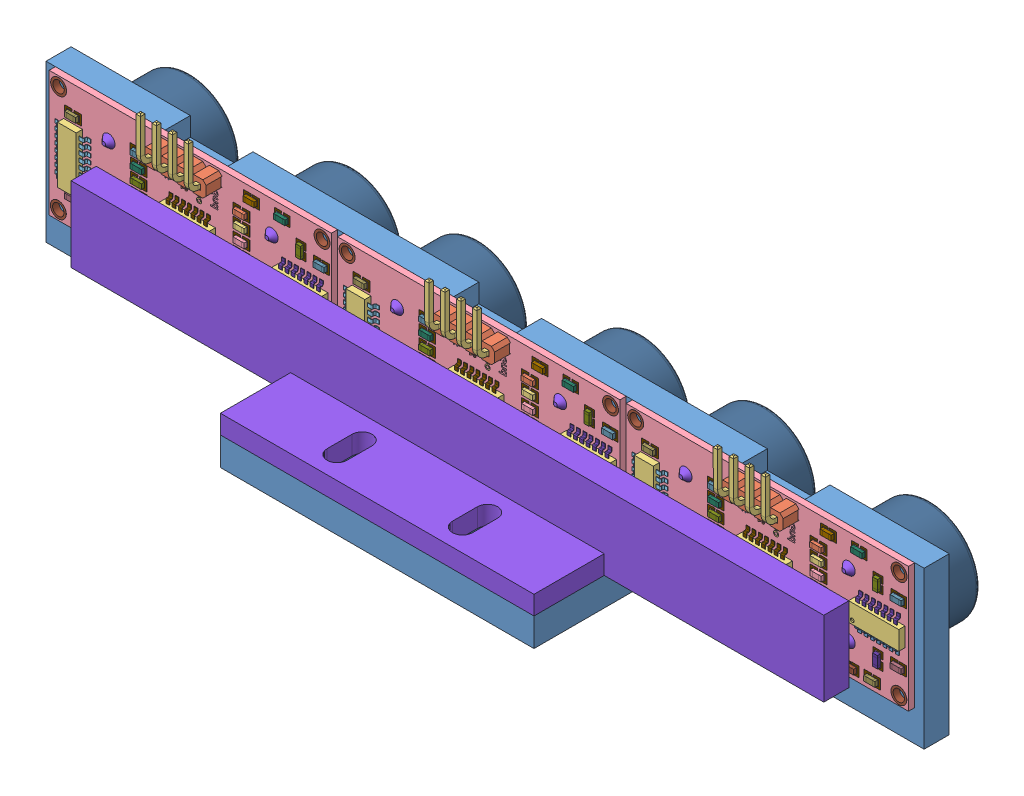
SolidWorks assembly Assem4, configuration Default. Lengths in mm.
Overall size (140 30.57 29.2).
188 component instances, 62 part files, 9 mates.
Components (placement in the parent):
- ga lap ultrasonic v5-1: ga lap ultrasonic v5 [Default] at (40.1597 76.4517 111.5417) size (140 25 21.2)
- HC-04HC-04-1: HC-04HC-04 [Default] at (54.2402 85.1585 116.5417) x (1 0 0) z (0 0 -1) size (45 25.57 17.46)
  - HC-04HC-04.stp-1: HC-04HC-04.stp [Default] at origin size (45 25.57 17.46)
    - HC-04Array.stp-1: HC-04Array.stp [Default] at origin size (10.16 2.54 2.54)
    - HC-04Array001.stp-1: HC-04Array001.stp [Default] at (0 0 1) size (8.32 7.52 6.46)
    - HC-04Placa.stp-1: HC-04Placa.stp [Default] at origin size (45 20 1)
    - HC-04Pad003.stp-1: HC-04Pad003.stp [Default] at (0 0 1) size (10.52 3.38 0.2)
    - HC-04Fillet.stp-1: HC-04Fillet.stp [Default] at (0 0 1) size (10.1 2.84 3)
    - HC-04Array002.stp-1: HC-04Array002.stp [Default] at origin size (9.62 2 1)
    - HC-04Array003.stp-1: HC-04Array003.stp [Default] at (0 0 1) size (28 12 0.8)
    - HC-04Fusion.stp-1: HC-04Fusion.stp [Default] at origin size (6 2 1)
    - HC-04Fillet001.stp-1: HC-04Fillet001.stp [Default] at (0 0 1) size (42 16 12)
    - HC-04Pad005.stp-1: HC-04Pad005.stp [Default] at (0 0 1) size (39.16 13 0.2)
    - HC-04Pad006.stp-1: HC-04Pad006.stp [Default] at (0 0 1) size (35.01 9.04 7)
    - HC-04Fusion001.stp-1: HC-04Fusion001.stp [Default] at (0 0 8) size (31 5 1.5)
    - HC-04Clone_of_Fusion002.stp-1: HC-04Clone_of_Fusion002.stp [Default] at (47.2 -5.5 12.6) size (13 13 0.15)
    - HC-04Clone_of_Fusion003.stp-1: HC-04Clone_of_Fusion003.stp [Default] at (21.2 -5.5 12.6) size (13 13 0.15)
    - HC-04Array005.stp-1: HC-04Array005.stp [Default] at origin size (9.62 2 1)
    - HC-04Array002002.stp-1: HC-04Array002002.stp [Default] at (-5.9 0.1 0.15) size (6.57 1.4 0.56)
    - HC-04Clone_of_Array002002.stp-1: HC-04Clone_of_Array002002.stp [Default] at (-23.9 0.1 0.15) size (6.57 1.4 0.56)
    - HC-04Array002003.stp-1: HC-04Array002003.stp [Default] at (-6.05 0 0.15) size (6.57 1.4 0.56)
    - HC-04Clone_of_Array002003.stp-1: HC-04Clone_of_Array002003.stp [Default] at (-24.05 0 0.15) size (6.57 1.4 0.56)
    - HC-04Integrados.stp-1: HC-04Integrados.stp [Default] at origin size (42.14 9 1)
    - HC-04ShapeString.stp-1: HC-04ShapeString.stp [Default] at (-3.2 -7 1.01) x (0 1 0) z (0 0 1) size (2.53 1.13 0.01)
    - HC-04ShapeString001.stp-1: HC-04ShapeString001.stp [Default] at (-0.6 -7 1.01) x (0 1 0) z (0 0 1) size (2.66 1.45 0.01)
    - HC-04ShapeString002.stp-1: HC-04ShapeString002.stp [Default] at (1.9 -7 1.01) x (0 1 0) z (0 0 1) size (3.21 1.16 0.01)
    - HC-04ShapeString003.stp-1: HC-04ShapeString003.stp [Default] at (4.5 -7 1.01) x (0 1 0) z (0 0 1) size (2.71 1.16 0.01)
    - HC-04ShapeString004.stp-1: HC-04ShapeString004.stp [Default] at (-19.5 -9.3 1.01) size (1.84 2.34 0.01)
    - HC-04ShapeString005.stp-1: HC-04ShapeString005.stp [Default] at (17.5 -9.3 1.01) size (1.82 2.34 0.01)
    - HC-04ShapeString006.stp-1: HC-04ShapeString006.stp [Default] at (-3 3.7 1.01) size (5.52 1.41 0.01)
    - HC-04Pad008.stp-1: HC-04Pad008.stp [Default] at (0 0 -0.01) size (44.56 19.6 1.02)
    - HC-04Scale004.stp-1: HC-04Scale004.stp [Default] at (-1.9 -21.5 -1.5) x (0 1 0) z (0 0 1) size (0.8 1.77 0.5)
    - HC-04Scale027.stp-1: HC-04Scale027.stp [Default] at (-1.9 -10.2323 -1.5) x (0 1 0) z (0 0 1) size (0.8 1.77 0.5)
    - HC-04Scale028.stp-1: HC-04Scale028.stp [Default] at (8.5984 -21.5 -1.5) x (0 1 0) z (0 0 1) size (0.8 1.77 0.5)
    - HC-04Scale029.stp-1: HC-04Scale029.stp [Default] at (8.5984 -19.5867 -1.5) x (0 1 0) z (0 0 1) size (0.8 1.77 0.5)
    - HC-04Scale030.stp-1: HC-04Scale030.stp [Default] at (8.5984 -17.5982 -1.5) x (0 1 0) z (0 0 1) size (0.8 1.77 0.5)
    - HC-04Scale031.stp-1: HC-04Scale031.stp [Default] at (8.5984 -15.6427 -1.5) x (0 1 0) z (0 0 1) size (0.8 1.77 0.5)
    - HC-04Scale032.stp-1: HC-04Scale032.stp [Default] at (8.5984 -11.6848 -1.5) x (0 1 0) z (0 0 1) size (0.8 1.77 0.5)
    - HC-04Scale033.stp-1: HC-04Scale033.stp [Default] at (-26.74 -2 -1.5) x (0 1 0) z (0 0 1) size (0.8 1.85 0.5)
    - HC-04Scale034.stp-1: HC-04Scale034.stp [Default] at (24.9371 -21.5 -1.5) x (0 1 0) z (0 0 1) size (0.8 1.77 0.5)
    - HC-04Scale035.stp-1: HC-04Scale035.stp [Default] at (24.9691 -19.5867 -1.5) x (0 1 0) z (0 0 1) size (0.8 1.77 0.5)
    - HC-04Scale036.stp-1: HC-04Scale036.stp [Default] at (24.9742 -17.5982 -1.5) x (0 1 0) z (0 0 1) size (0.8 1.77 0.5)
    - HC-04Scale037.stp-1: HC-04Scale037.stp [Default] at (-10.4013 -2 -1.5) x (0 1 0) z (0 0 1) size (0.8 1.85 0.5)
    - HC-04Scale038.stp-1: HC-04Scale038.stp [Default] at (-10.4013 -3.9266 -1.5) x (0 1 0) z (0 0 1) size (0.8 1.85 0.5)
    - HC-04Scale039.stp-1: HC-04Scale039.stp [Default] at (-10.4013 -0.0734 -1.5) x (0 1 0) z (0 0 1) size (0.8 1.85 0.5)
    - HC-04Scale040.stp-1: HC-04Scale040.stp [Default] at (24.9742 -9.855 -1.5) x (0 1 0) z (0 0 1) size (0.8 1.77 0.5)
    - HC-04Scale041.stp-1: HC-04Scale041.stp [Default] at (26.5673 -24.0564 -1.5) x (0 1 0) z (0 0 1) size (0.8 1.77 0.5)
    - HC-04Scale042.stp-1: HC-04Scale042.stp [Default] at (26.5673 -7.3333 -1.5) x (0 1 0) z (0 0 1) size (0.8 1.77 0.5)
    - HC-04Scale043.stp-1: HC-04Scale043.stp [Default] at (30.1435 -7.3333 -1.5) x (0 1 0) z (0 0 1) size (0.8 1.77 0.5)
    - HC-04Scale044.stp-1: HC-04Scale044.stp [Default] at (33.5459 -7.3333 -1.5) x (0 1 0) z (0 0 1) size (0.8 1.77 0.5)
    - HC-04Scale045.stp-1: HC-04Scale045.stp [Default] at (37.7181 -11.1827 -1.5) x (0 1 0) z (0 0 1) size (0.8 1.77 0.5)
    - HC-04Scale046.stp-1: HC-04Scale046.stp [Default] at (37.7181 -20.5932 -1.5) x (0 1 0) z (0 0 1) size (0.8 1.77 0.5)
    - HC-04Scale047.stp-1: HC-04Scale047.stp [Default] at (-3.9042 -12.3288 -1.5) x (0 1 0) z (0 0 1) size (0.8 1.85 0.5)
    - HC-04Scale048.stp-1: HC-04Scale048.stp [Default] at (13.5402 13.2894 -1.5) size (0.8 1.85 0.5)
    - HC-04Scale049.stp-1: HC-04Scale049.stp [Default] at (13.5402 23.7909 -1.5) size (0.8 1.85 0.5)
    - HC-04Pad009.stp-1: HC-04Pad009.stp [Default] x (1 0 0) z (0 0 -1) size (42.21 18.43 0.01)
    - HC-04ShapeString007.stp-1: HC-04ShapeString007.stp [Default] at (-3.2 -7 -0.1) x (0 1 0) z (0 0 1) size (2.53 1.13 0.01)
    - HC-04ShapeString008.stp-1: HC-04ShapeString008.stp [Default] at (-0.6 -7 -0.1) x (0 1 0) z (0 0 1) size (2.66 1.45 0.01)
    - HC-04ShapeString009.stp-1: HC-04ShapeString009.stp [Default] at (1.9 -7 -0.1) x (0 1 0) z (0 0 1) size (3.21 1.16 0.01)
    - HC-04ShapeString010.stp-1: HC-04ShapeString010.stp [Default] at (4.5 -7 -0.1) x (0 1 0) z (0 0 1) size (2.71 1.16 0.01)
    - HC-04Fusion002.stp-1: HC-04Fusion002.stp [Default] at origin size (5.7 7.57 0.56)
    - HC-04ShapeString011.stp-1: HC-04ShapeString011.stp [Default] at (-17.5 8.4 1.1) size (7.91 1.16 0.01)
    - HC-04ShapeString012.stp-1: HC-04ShapeString012.stp [Default] at (-7.5 8 -0.1) x (-1 0 0) z (0 0 -1) size (7.91 1.16 0.01)
- HC-04HC-04-2: HC-04HC-04 [Default] at (100.2402 85.1585 116.5417) x (1 0 0) z (0 0 -1) size (45 25.57 17.46)
  - HC-04HC-04.stp-1: HC-04HC-04.stp [Default] at origin size (45 25.57 17.46)
    - HC-04Array.stp-1: HC-04Array.stp [Default] at origin size (10.16 2.54 2.54)
    - HC-04Array001.stp-1: HC-04Array001.stp [Default] at (0 0 1) size (8.32 7.52 6.46)
    - HC-04Placa.stp-1: HC-04Placa.stp [Default] at origin size (45 20 1)
    - HC-04Pad003.stp-1: HC-04Pad003.stp [Default] at (0 0 1) size (10.52 3.38 0.2)
    - HC-04Fillet.stp-1: HC-04Fillet.stp [Default] at (0 0 1) size (10.1 2.84 3)
    - HC-04Array002.stp-1: HC-04Array002.stp [Default] at origin size (9.62 2 1)
    - HC-04Array003.stp-1: HC-04Array003.stp [Default] at (0 0 1) size (28 12 0.8)
    - HC-04Fusion.stp-1: HC-04Fusion.stp [Default] at origin size (6 2 1)
    - HC-04Fillet001.stp-1: HC-04Fillet001.stp [Default] at (0 0 1) size (42 16 12)
    - HC-04Pad005.stp-1: HC-04Pad005.stp [Default] at (0 0 1) size (39.16 13 0.2)
    - HC-04Pad006.stp-1: HC-04Pad006.stp [Default] at (0 0 1) size (35.01 9.04 7)
    - HC-04Fusion001.stp-1: HC-04Fusion001.stp [Default] at (0 0 8) size (31 5 1.5)
    - HC-04Clone_of_Fusion002.stp-1: HC-04Clone_of_Fusion002.stp [Default] at (47.2 -5.5 12.6) size (13 13 0.15)
    - HC-04Clone_of_Fusion003.stp-1: HC-04Clone_of_Fusion003.stp [Default] at (21.2 -5.5 12.6) size (13 13 0.15)
    - HC-04Array005.stp-1: HC-04Array005.stp [Default] at origin size (9.62 2 1)
    - HC-04Array002002.stp-1: HC-04Array002002.stp [Default] at (-5.9 0.1 0.15) size (6.57 1.4 0.56)
    - HC-04Clone_of_Array002002.stp-1: HC-04Clone_of_Array002002.stp [Default] at (-23.9 0.1 0.15) size (6.57 1.4 0.56)
    - HC-04Array002003.stp-1: HC-04Array002003.stp [Default] at (-6.05 0 0.15) size (6.57 1.4 0.56)
    - HC-04Clone_of_Array002003.stp-1: HC-04Clone_of_Array002003.stp [Default] at (-24.05 0 0.15) size (6.57 1.4 0.56)
    - HC-04Integrados.stp-1: HC-04Integrados.stp [Default] at origin size (42.14 9 1)
    - HC-04ShapeString.stp-1: HC-04ShapeString.stp [Default] at (-3.2 -7 1.01) x (0 1 0) z (0 0 1) size (2.53 1.13 0.01)
    - HC-04ShapeString001.stp-1: HC-04ShapeString001.stp [Default] at (-0.6 -7 1.01) x (0 1 0) z (0 0 1) size (2.66 1.45 0.01)
    - HC-04ShapeString002.stp-1: HC-04ShapeString002.stp [Default] at (1.9 -7 1.01) x (0 1 0) z (0 0 1) size (3.21 1.16 0.01)
    - HC-04ShapeString003.stp-1: HC-04ShapeString003.stp [Default] at (4.5 -7 1.01) x (0 1 0) z (0 0 1) size (2.71 1.16 0.01)
    - HC-04ShapeString004.stp-1: HC-04ShapeString004.stp [Default] at (-19.5 -9.3 1.01) size (1.84 2.34 0.01)
    - HC-04ShapeString005.stp-1: HC-04ShapeString005.stp [Default] at (17.5 -9.3 1.01) size (1.82 2.34 0.01)
    - HC-04ShapeString006.stp-1: HC-04ShapeString006.stp [Default] at (-3 3.7 1.01) size (5.52 1.41 0.01)
    - HC-04Pad008.stp-1: HC-04Pad008.stp [Default] at (0 0 -0.01) size (44.56 19.6 1.02)
    - HC-04Scale004.stp-1: HC-04Scale004.stp [Default] at (-1.9 -21.5 -1.5) x (0 1 0) z (0 0 1) size (0.8 1.77 0.5)
    - HC-04Scale027.stp-1: HC-04Scale027.stp [Default] at (-1.9 -10.2323 -1.5) x (0 1 0) z (0 0 1) size (0.8 1.77 0.5)
    - HC-04Scale028.stp-1: HC-04Scale028.stp [Default] at (8.5984 -21.5 -1.5) x (0 1 0) z (0 0 1) size (0.8 1.77 0.5)
    - HC-04Scale029.stp-1: HC-04Scale029.stp [Default] at (8.5984 -19.5867 -1.5) x (0 1 0) z (0 0 1) size (0.8 1.77 0.5)
    - HC-04Scale030.stp-1: HC-04Scale030.stp [Default] at (8.5984 -17.5982 -1.5) x (0 1 0) z (0 0 1) size (0.8 1.77 0.5)
    - HC-04Scale031.stp-1: HC-04Scale031.stp [Default] at (8.5984 -15.6427 -1.5) x (0 1 0) z (0 0 1) size (0.8 1.77 0.5)
    - HC-04Scale032.stp-1: HC-04Scale032.stp [Default] at (8.5984 -11.6848 -1.5) x (0 1 0) z (0 0 1) size (0.8 1.77 0.5)
    - HC-04Scale033.stp-1: HC-04Scale033.stp [Default] at (-26.74 -2 -1.5) x (0 1 0) z (0 0 1) size (0.8 1.85 0.5)
    - HC-04Scale034.stp-1: HC-04Scale034.stp [Default] at (24.9371 -21.5 -1.5) x (0 1 0) z (0 0 1) size (0.8 1.77 0.5)
    - HC-04Scale035.stp-1: HC-04Scale035.stp [Default] at (24.9691 -19.5867 -1.5) x (0 1 0) z (0 0 1) size (0.8 1.77 0.5)
    - HC-04Scale036.stp-1: HC-04Scale036.stp [Default] at (24.9742 -17.5982 -1.5) x (0 1 0) z (0 0 1) size (0.8 1.77 0.5)
    - HC-04Scale037.stp-1: HC-04Scale037.stp [Default] at (-10.4013 -2 -1.5) x (0 1 0) z (0 0 1) size (0.8 1.85 0.5)
    - HC-04Scale038.stp-1: HC-04Scale038.stp [Default] at (-10.4013 -3.9266 -1.5) x (0 1 0) z (0 0 1) size (0.8 1.85 0.5)
    - HC-04Scale039.stp-1: HC-04Scale039.stp [Default] at (-10.4013 -0.0734 -1.5) x (0 1 0) z (0 0 1) size (0.8 1.85 0.5)
    - HC-04Scale040.stp-1: HC-04Scale040.stp [Default] at (24.9742 -9.855 -1.5) x (0 1 0) z (0 0 1) size (0.8 1.77 0.5)
    - HC-04Scale041.stp-1: HC-04Scale041.stp [Default] at (26.5673 -24.0564 -1.5) x (0 1 0) z (0 0 1) size (0.8 1.77 0.5)
    - HC-04Scale042.stp-1: HC-04Scale042.stp [Default] at (26.5673 -7.3333 -1.5) x (0 1 0) z (0 0 1) size (0.8 1.77 0.5)
    - HC-04Scale043.stp-1: HC-04Scale043.stp [Default] at (30.1435 -7.3333 -1.5) x (0 1 0) z (0 0 1) size (0.8 1.77 0.5)
    - HC-04Scale044.stp-1: HC-04Scale044.stp [Default] at (33.5459 -7.3333 -1.5) x (0 1 0) z (0 0 1) size (0.8 1.77 0.5)
    - HC-04Scale045.stp-1: HC-04Scale045.stp [Default] at (37.7181 -11.1827 -1.5) x (0 1 0) z (0 0 1) size (0.8 1.77 0.5)
    - HC-04Scale046.stp-1: HC-04Scale046.stp [Default] at (37.7181 -20.5932 -1.5) x (0 1 0) z (0 0 1) size (0.8 1.77 0.5)
    - HC-04Scale047.stp-1: HC-04Scale047.stp [Default] at (-3.9042 -12.3288 -1.5) x (0 1 0) z (0 0 1) size (0.8 1.85 0.5)
    - HC-04Scale048.stp-1: HC-04Scale048.stp [Default] at (13.5402 13.2894 -1.5) size (0.8 1.85 0.5)
    - HC-04Scale049.stp-1: HC-04Scale049.stp [Default] at (13.5402 23.7909 -1.5) size (0.8 1.85 0.5)
    - HC-04Pad009.stp-1: HC-04Pad009.stp [Default] x (1 0 0) z (0 0 -1) size (42.21 18.43 0.01)
    - HC-04ShapeString007.stp-1: HC-04ShapeString007.stp [Default] at (-3.2 -7 -0.1) x (0 1 0) z (0 0 1) size (2.53 1.13 0.01)
    - HC-04ShapeString008.stp-1: HC-04ShapeString008.stp [Default] at (-0.6 -7 -0.1) x (0 1 0) z (0 0 1) size (2.66 1.45 0.01)
    - HC-04ShapeString009.stp-1: HC-04ShapeString009.stp [Default] at (1.9 -7 -0.1) x (0 1 0) z (0 0 1) size (3.21 1.16 0.01)
    - HC-04ShapeString010.stp-1: HC-04ShapeString010.stp [Default] at (4.5 -7 -0.1) x (0 1 0) z (0 0 1) size (2.71 1.16 0.01)
    - HC-04Fusion002.stp-1: HC-04Fusion002.stp [Default] at origin size (5.7 7.57 0.56)
    - HC-04ShapeString011.stp-1: HC-04ShapeString011.stp [Default] at (-17.5 8.4 1.1) size (7.91 1.16 0.01)
    - HC-04ShapeString012.stp-1: HC-04ShapeString012.stp [Default] at (-7.5 8 -0.1) x (-1 0 0) z (0 0 -1) size (7.91 1.16 0.01)
- HC-04HC-04-3: HC-04HC-04 [Default] at (8.2402 85.1585 116.5417) x (1 0 0) z (0 0 -1) size (45 25.57 17.46)
  - HC-04HC-04.stp-1: HC-04HC-04.stp [Default] at origin size (45 25.57 17.46)
    - HC-04Array.stp-1: HC-04Array.stp [Default] at origin size (10.16 2.54 2.54)
    - HC-04Array001.stp-1: HC-04Array001.stp [Default] at (0 0 1) size (8.32 7.52 6.46)
    - HC-04Placa.stp-1: HC-04Placa.stp [Default] at origin size (45 20 1)
    - HC-04Pad003.stp-1: HC-04Pad003.stp [Default] at (0 0 1) size (10.52 3.38 0.2)
    - HC-04Fillet.stp-1: HC-04Fillet.stp [Default] at (0 0 1) size (10.1 2.84 3)
    - HC-04Array002.stp-1: HC-04Array002.stp [Default] at origin size (9.62 2 1)
    - HC-04Array003.stp-1: HC-04Array003.stp [Default] at (0 0 1) size (28 12 0.8)
    - HC-04Fusion.stp-1: HC-04Fusion.stp [Default] at origin size (6 2 1)
    - HC-04Fillet001.stp-1: HC-04Fillet001.stp [Default] at (0 0 1) size (42 16 12)
    - HC-04Pad005.stp-1: HC-04Pad005.stp [Default] at (0 0 1) size (39.16 13 0.2)
    - HC-04Pad006.stp-1: HC-04Pad006.stp [Default] at (0 0 1) size (35.01 9.04 7)
    - HC-04Fusion001.stp-1: HC-04Fusion001.stp [Default] at (0 0 8) size (31 5 1.5)
    - HC-04Clone_of_Fusion002.stp-1: HC-04Clone_of_Fusion002.stp [Default] at (47.2 -5.5 12.6) size (13 13 0.15)
    - HC-04Clone_of_Fusion003.stp-1: HC-04Clone_of_Fusion003.stp [Default] at (21.2 -5.5 12.6) size (13 13 0.15)
    - HC-04Array005.stp-1: HC-04Array005.stp [Default] at origin size (9.62 2 1)
    - HC-04Array002002.stp-1: HC-04Array002002.stp [Default] at (-5.9 0.1 0.15) size (6.57 1.4 0.56)
    - HC-04Clone_of_Array002002.stp-1: HC-04Clone_of_Array002002.stp [Default] at (-23.9 0.1 0.15) size (6.57 1.4 0.56)
    - HC-04Array002003.stp-1: HC-04Array002003.stp [Default] at (-6.05 0 0.15) size (6.57 1.4 0.56)
    - HC-04Clone_of_Array002003.stp-1: HC-04Clone_of_Array002003.stp [Default] at (-24.05 0 0.15) size (6.57 1.4 0.56)
    - HC-04Integrados.stp-1: HC-04Integrados.stp [Default] at origin size (42.14 9 1)
    - HC-04ShapeString.stp-1: HC-04ShapeString.stp [Default] at (-3.2 -7 1.01) x (0 1 0) z (0 0 1) size (2.53 1.13 0.01)
    - HC-04ShapeString001.stp-1: HC-04ShapeString001.stp [Default] at (-0.6 -7 1.01) x (0 1 0) z (0 0 1) size (2.66 1.45 0.01)
    - HC-04ShapeString002.stp-1: HC-04ShapeString002.stp [Default] at (1.9 -7 1.01) x (0 1 0) z (0 0 1) size (3.21 1.16 0.01)
    - HC-04ShapeString003.stp-1: HC-04ShapeString003.stp [Default] at (4.5 -7 1.01) x (0 1 0) z (0 0 1) size (2.71 1.16 0.01)
    - HC-04ShapeString004.stp-1: HC-04ShapeString004.stp [Default] at (-19.5 -9.3 1.01) size (1.84 2.34 0.01)
    - HC-04ShapeString005.stp-1: HC-04ShapeString005.stp [Default] at (17.5 -9.3 1.01) size (1.82 2.34 0.01)
    - HC-04ShapeString006.stp-1: HC-04ShapeString006.stp [Default] at (-3 3.7 1.01) size (5.52 1.41 0.01)
    - HC-04Pad008.stp-1: HC-04Pad008.stp [Default] at (0 0 -0.01) size (44.56 19.6 1.02)
    - HC-04Scale004.stp-1: HC-04Scale004.stp [Default] at (-1.9 -21.5 -1.5) x (0 1 0) z (0 0 1) size (0.8 1.77 0.5)
    - HC-04Scale027.stp-1: HC-04Scale027.stp [Default] at (-1.9 -10.2323 -1.5) x (0 1 0) z (0 0 1) size (0.8 1.77 0.5)
    - HC-04Scale028.stp-1: HC-04Scale028.stp [Default] at (8.5984 -21.5 -1.5) x (0 1 0) z (0 0 1) size (0.8 1.77 0.5)
    - HC-04Scale029.stp-1: HC-04Scale029.stp [Default] at (8.5984 -19.5867 -1.5) x (0 1 0) z (0 0 1) size (0.8 1.77 0.5)
    - HC-04Scale030.stp-1: HC-04Scale030.stp [Default] at (8.5984 -17.5982 -1.5) x (0 1 0) z (0 0 1) size (0.8 1.77 0.5)
    - HC-04Scale031.stp-1: HC-04Scale031.stp [Default] at (8.5984 -15.6427 -1.5) x (0 1 0) z (0 0 1) size (0.8 1.77 0.5)
    - HC-04Scale032.stp-1: HC-04Scale032.stp [Default] at (8.5984 -11.6848 -1.5) x (0 1 0) z (0 0 1) size (0.8 1.77 0.5)
    - HC-04Scale033.stp-1: HC-04Scale033.stp [Default] at (-26.74 -2 -1.5) x (0 1 0) z (0 0 1) size (0.8 1.85 0.5)
    - HC-04Scale034.stp-1: HC-04Scale034.stp [Default] at (24.9371 -21.5 -1.5) x (0 1 0) z (0 0 1) size (0.8 1.77 0.5)
    - HC-04Scale035.stp-1: HC-04Scale035.stp [Default] at (24.9691 -19.5867 -1.5) x (0 1 0) z (0 0 1) size (0.8 1.77 0.5)
    - HC-04Scale036.stp-1: HC-04Scale036.stp [Default] at (24.9742 -17.5982 -1.5) x (0 1 0) z (0 0 1) size (0.8 1.77 0.5)
    - HC-04Scale037.stp-1: HC-04Scale037.stp [Default] at (-10.4013 -2 -1.5) x (0 1 0) z (0 0 1) size (0.8 1.85 0.5)
    - HC-04Scale038.stp-1: HC-04Scale038.stp [Default] at (-10.4013 -3.9266 -1.5) x (0 1 0) z (0 0 1) size (0.8 1.85 0.5)
    - HC-04Scale039.stp-1: HC-04Scale039.stp [Default] at (-10.4013 -0.0734 -1.5) x (0 1 0) z (0 0 1) size (0.8 1.85 0.5)
    - HC-04Scale040.stp-1: HC-04Scale040.stp [Default] at (24.9742 -9.855 -1.5) x (0 1 0) z (0 0 1) size (0.8 1.77 0.5)
    - HC-04Scale041.stp-1: HC-04Scale041.stp [Default] at (26.5673 -24.0564 -1.5) x (0 1 0) z (0 0 1) size (0.8 1.77 0.5)
    - HC-04Scale042.stp-1: HC-04Scale042.stp [Default] at (26.5673 -7.3333 -1.5) x (0 1 0) z (0 0 1) size (0.8 1.77 0.5)
    - HC-04Scale043.stp-1: HC-04Scale043.stp [Default] at (30.1435 -7.3333 -1.5) x (0 1 0) z (0 0 1) size (0.8 1.77 0.5)
    - HC-04Scale044.stp-1: HC-04Scale044.stp [Default] at (33.5459 -7.3333 -1.5) x (0 1 0) z (0 0 1) size (0.8 1.77 0.5)
    - HC-04Scale045.stp-1: HC-04Scale045.stp [Default] at (37.7181 -11.1827 -1.5) x (0 1 0) z (0 0 1) size (0.8 1.77 0.5)
    - HC-04Scale046.stp-1: HC-04Scale046.stp [Default] at (37.7181 -20.5932 -1.5) x (0 1 0) z (0 0 1) size (0.8 1.77 0.5)
    - HC-04Scale047.stp-1: HC-04Scale047.stp [Default] at (-3.9042 -12.3288 -1.5) x (0 1 0) z (0 0 1) size (0.8 1.85 0.5)
    - HC-04Scale048.stp-1: HC-04Scale048.stp [Default] at (13.5402 13.2894 -1.5) size (0.8 1.85 0.5)
    - HC-04Scale049.stp-1: HC-04Scale049.stp [Default] at (13.5402 23.7909 -1.5) size (0.8 1.85 0.5)
    - HC-04Pad009.stp-1: HC-04Pad009.stp [Default] x (1 0 0) z (0 0 -1) size (42.21 18.43 0.01)
    - HC-04ShapeString007.stp-1: HC-04ShapeString007.stp [Default] at (-3.2 -7 -0.1) x (0 1 0) z (0 0 1) size (2.53 1.13 0.01)
    - HC-04ShapeString008.stp-1: HC-04ShapeString008.stp [Default] at (-0.6 -7 -0.1) x (0 1 0) z (0 0 1) size (2.66 1.45 0.01)
    - HC-04ShapeString009.stp-1: HC-04ShapeString009.stp [Default] at (1.9 -7 -0.1) x (0 1 0) z (0 0 1) size (3.21 1.16 0.01)
    - HC-04ShapeString010.stp-1: HC-04ShapeString010.stp [Default] at (4.5 -7 -0.1) x (0 1 0) z (0 0 1) size (2.71 1.16 0.01)
    - HC-04Fusion002.stp-1: HC-04Fusion002.stp [Default] at origin size (5.7 7.57 0.56)
    - HC-04ShapeString011.stp-1: HC-04ShapeString011.stp [Default] at (-17.5 8.4 1.1) size (7.91 1.16 0.01)
    - HC-04ShapeString012.stp-1: HC-04ShapeString012.stp [Default] at (-7.5 8 -0.1) x (-1 0 0) z (0 0 -1) size (7.91 1.16 0.01)
- chot giu-1: chot giu [Default] at (58.0076 52.0621 117.5417) size (120 12 15.2)
Mates (geometry in assembly coordinates):
- Concentric1: concentric anti-aligned: cylinder of ga lap ultrasonic v5-1 through (67.2402 85.1586 115.5417) axis (0 0 -1) radius 8.5; cylinder of HC-04HC-04-1/HC-04HC-04.stp-1/HC-04Fillet001.stp-1 through (67.2402 85.1586 115.5417) axis (0 0 1) radius 8
- Coincident1: coincident anti-aligned: plane of ga lap ultrasonic v5-1 through (40.1597 76.4517 115.5417) normal (0 0 1); plane of HC-04HC-04-1/HC-04HC-04.stp-1/HC-04Placa.stp-1 through (31.7402 75.1585 115.5417) normal (0 0 -1)
- Concentric2: concentric anti-aligned: cylinder of ga lap ultrasonic v5-1 through (87.2402 85.1586 115.5417) axis (0 0 -1) radius 8.5; cylinder of HC-04HC-04-2/HC-04HC-04.stp-1/HC-04Fillet001.stp-1 through (87.2402 85.1586 115.5417) axis (0 0 1) radius 8
- Coincident2: coincident anti-aligned: plane of ga lap ultrasonic v5-1 through (40.1597 76.4517 115.5417) normal (0 0 1); plane of HC-04HC-04-2/HC-04HC-04.stp-1/HC-04Placa.stp-1 through (77.7402 75.1585 115.5417) normal (0 0 -1)
- Concentric3: concentric anti-aligned: cylinder of ga lap ultrasonic v5-1 through (-4.7598 85.1586 115.5417) axis (0 0 -1) radius 8.5; cylinder of HC-04HC-04-3/HC-04HC-04.stp-1/HC-04Fillet001.stp-1 through (-4.7598 85.1586 115.5417) axis (0 0 1) radius 8
- Coincident3: coincident anti-aligned: plane of ga lap ultrasonic v5-1 through (40.1597 76.4517 115.5417) normal (0 0 1); plane of HC-04HC-04-3/HC-04HC-04.stp-1/HC-04Placa.stp-1 through (-14.2598 75.1585 115.5417) normal (0 0 -1)
- Coincident5: coincident anti-aligned: plane of ga lap ultrasonic v5-1 through (79.2402 74.6586 132.7417) normal (0 1 0); plane of chot giu-1 through (-5.7598 74.6586 121.5417) normal (0 -1 0)
- Coincident6: coincident aligned: plane of ga lap ultrasonic v5-1 through (42.6402 70.1586 129.1417) normal (1 0 0); plane of chot giu-1 through (42.6402 74.6586 117.5417) normal (1 0 0)
- Coincident7: coincident anti-aligned: plane of HC-04HC-04-1/HC-04HC-04.stp-1/HC-04Integrados.stp-1 through (68.1968 83.6585 117.5417) normal (0 0 1); plane of chot giu-1 through (58.0076 52.0621 117.5417) normal (0 0 -1)
